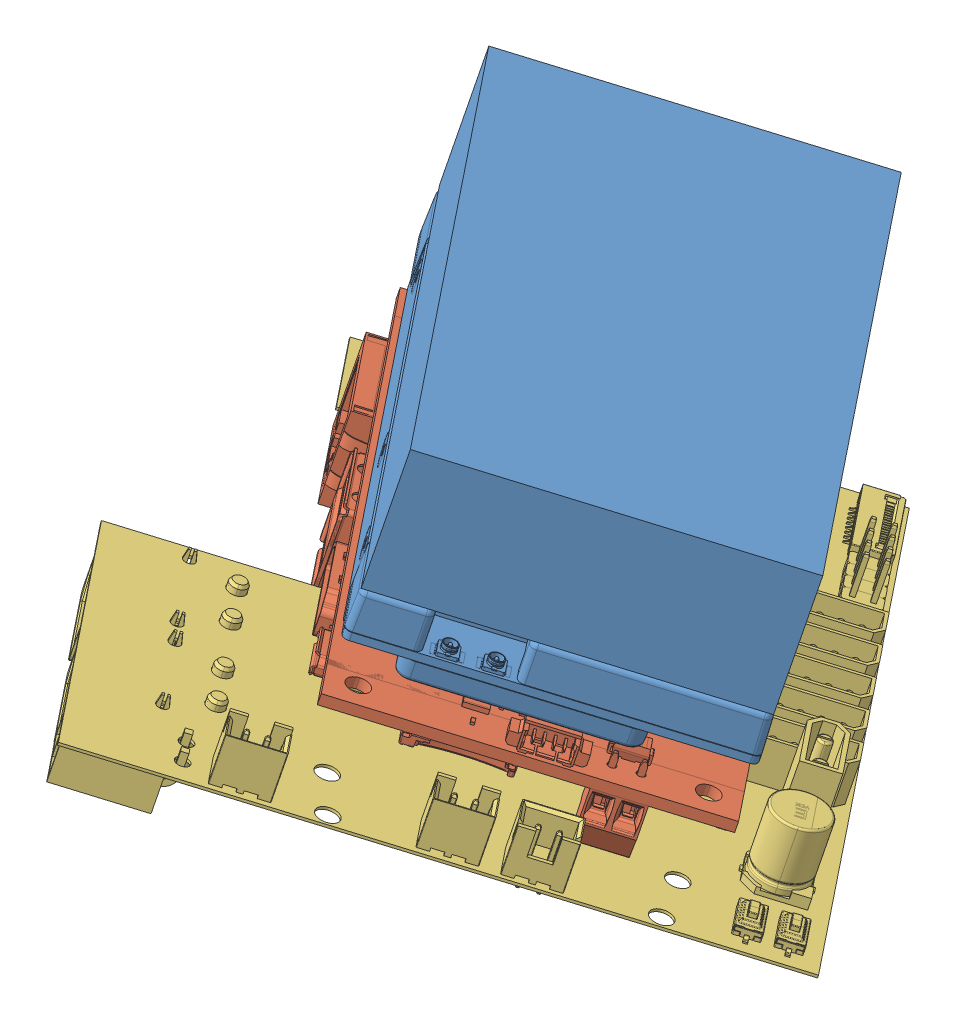
SolidWorks assembly 电路, configuration 默认. Lengths in mm.
Overall size (135.66 81.1 136.29).
3 component instances, 3 part files, 6 mates.
Components (placement in the parent):
- TX2-1: TX2 [默认] at (66.6739 -13.371 209.1651) x (-0.629094 -0.048866 -0.775792) z (0.186421 0.959412 -0.211602) size (87.07 50.04 32.13)
- 9003-1: 9003 [默认] at (15.6894 -27.7493 144.427) x (0.629094 0.048866 0.775792) z (-0.186421 -0.959412 0.211602) size (96.22 72.67 50.58)
- Main-1: Main [默认] at (20.5563 -29.3993 193.2183) x (0.629094 0.048866 0.775792) z (0.186421 0.959412 -0.211602) size (100 91.07 21.61)
Mates (geometry in assembly coordinates):
- 同心3: concentric: cylinder of ? through (17.0771 -16.7162 147.7627) axis (0.186421 0.959412 -0.211602) radius 1.8; cylinder of ? through (15.5223 -24.7181 149.5275) axis (0.186421 0.959412 -0.211602) radius 1.6
- 平行2: parallel: plane of ? through (7.6051 -0.6901 205.35) normal (-0.754644 0.277742 0.594451); plane of ? through (-22.0061 -13.6731 174.1078) normal (-0.754644 0.277742 0.594451)
- 距离2: distance = 8 mm: plane of assembly; plane of assembly; plane of TX2-1 through (66.6739 -13.371 209.1651) normal (-0.186421 -0.959412 0.211602); plane of 9003-1 through (15.9877 -26.2137 144.0883) normal (0.186421 0.959412 -0.211602)
- 同心4: concentric: cylinder of ? through (65.2208 -20.8577 210.815) axis (0.186421 0.959412 -0.211602) radius 1.6; cylinder of Main-1 through (62.7583 -33.5308 213.6102) axis (-0.186421 -0.959412 0.211602) radius 1.6
- 同心5: concentric: cylinder of ? through (15.5223 -24.7181 149.5275) axis (0.186421 0.959412 -0.211602) radius 1.6; cylinder of Main-1 through (13.0598 -37.3912 152.3226) axis (-0.186421 -0.959412 0.211602) radius 1.6
- 距离3: distance = 11 mm: plane of assembly; plane of assembly; plane of 9003-1 through (15.6894 -27.7493 144.427) normal (-0.186421 -0.959412 0.211602); plane of Main-1 through (-30.4465 -23.9002 173.2178) normal (0.186421 0.959412 -0.211602)
